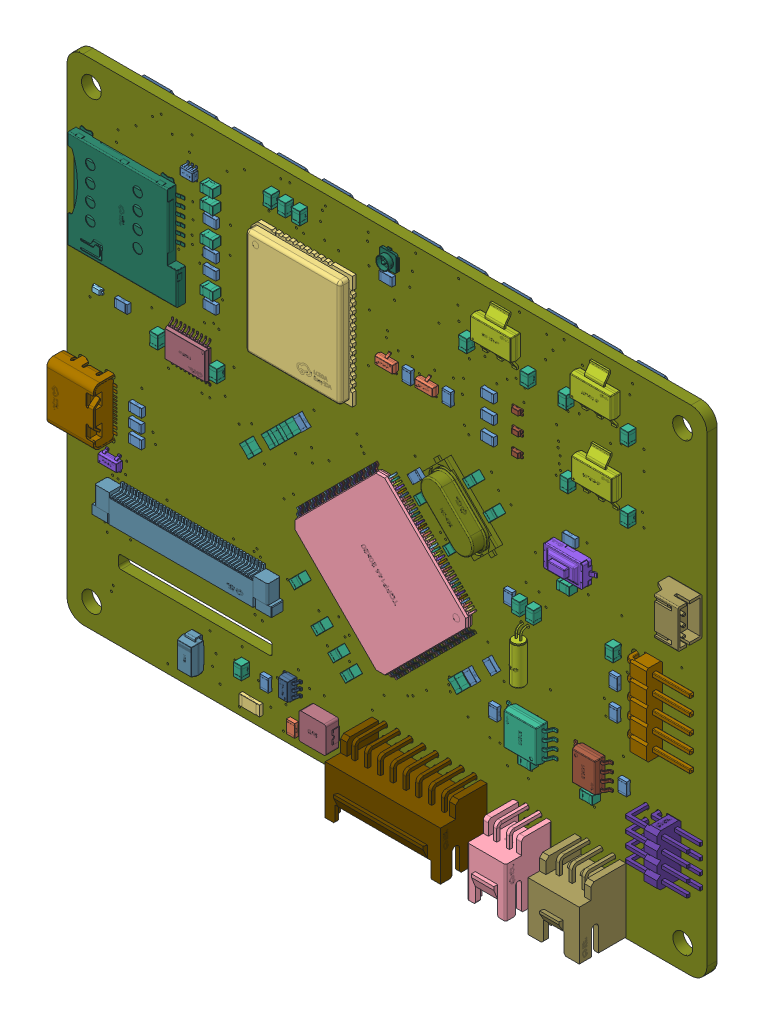
SolidWorks assembly steeringWheel_PCBA_v2.4, configuration 默认. Lengths in mm.
Overall size (100.05 77.22 11.5).
501 component instances, 178 part files, 0 mates.
Components (placement in the parent):
- steeringWheel_PCBA_v2.4.step-1: steeringWheel_PCBA_v2.4.step [默认] at origin size (100.05 77.22 11.5)
  - R5.step-1: R5.step [默认] at (22.8608 -12.1785 1.6001) size (2 1.3 0.61)
    - R0805.step-1: R0805.step [默认] at origin size (2 1.3 0.61)
      - COMPOUND.step-1: COMPOUND.step [默认] at origin size (2 1.3 0.61)
  - R17.step-1: R17.step [默认] at (22.8608 -19.1262 1.6001) size (2 1.3 0.61)
    - R0805.step-1: R0805.step [默认] at origin size (2 1.3 0.61)
      - COMPOUND.step-1: COMPOUND.step [默认] at origin size (2 1.3 0.61)
  - R16.step-1: R16.step [默认] at (22.8608 -16.8013 1.6001) size (2 1.3 0.61)
    - R0805.step-1: R0805.step [默认] at origin size (2 1.3 0.61)
      - COMPOUND.step-1: COMPOUND.step [默认] at origin size (2 1.3 0.61)
  - R12.step-1: R12.step [默认] at (11.1969 -45.6947 1.6001) x (-1 0 0) z (0 0 1) size (2 1.3 0.61)
    - R0805.step-1: R0805.step [默认] at origin size (2 1.3 0.61)
      - COMPOUND.step-1: COMPOUND.step [默认] at origin size (2 1.3 0.61)
  - R13.step-1: R13.step [默认] at (11.2213 -47.7775 1.6001) x (-1 0 0) z (0 0 1) size (2 1.3 0.61)
    - R0805.step-1: R0805.step [默认] at origin size (2 1.3 0.61)
      - COMPOUND.step-1: COMPOUND.step [默认] at origin size (2 1.3 0.61)
  - R19.step-1: R19.step [默认] at (67.1323 -56.4887 1.6001) x (0 -1 0) z (0 0 1) size (2 1.3 0.61)
    - R0805.step-1: R0805.step [默认] at origin size (2 1.3 0.61)
      - COMPOUND.step-1: COMPOUND.step [默认] at origin size (2 1.3 0.61)
  - R39.step-1: R39.step [默认] at (54.8869 -30.762 1.6001) x (-0.707107 -0.707107 0) z (0 0 1) size (2 1.3 0.61)
    - R0805.step-1: R0805.step [默认] at origin size (2 1.3 0.61)
      - COMPOUND.step-1: COMPOUND.step [默认] at origin size (2 1.3 0.61)
  - R40.step-1: R40.step [默认] at (63.5255 -53.4925 1.6001) x (0.707107 -0.707107 0) z (0 0 1) size (2 1.3 0.61)
    - R0805.step-1: R0805.step [默认] at origin size (2 1.3 0.61)
      - COMPOUND.step-1: COMPOUND.step [默认] at origin size (2 1.3 0.61)
  - R1.step-1: R1.step [默认] at (78.9688 -27.3051 1.6001) size (2 1.3 0.61)
    - R0805.step-1: R0805.step [默认] at origin size (2 1.3 0.61)
      - COMPOUND.step-1: COMPOUND.step [默认] at origin size (2 1.3 0.61)
  - R8.step-1: R8.step [默认] at (31.3945 -70.4343 1.6001) x (0 1 0) z (0 0 1) size (2 1.3 0.61)
    - R0805.step-1: R0805.step [默认] at origin size (2 1.3 0.61)
      - COMPOUND.step-1: COMPOUND.step [默认] at origin size (2 1.3 0.61)
  - R9.step-1: R9.step [默认] at (22.8608 -23.749 1.6001) size (2 1.3 0.61)
    - R0805.step-1: R0805.step [默认] at origin size (2 1.3 0.61)
      - COMPOUND.step-1: COMPOUND.step [默认] at origin size (2 1.3 0.61)
  - R41.step-1: R41.step [默认] at (66.2475 -19.8882 1.6001) x (-1 0 0) z (0 0 1) size (2 1.3 0.61)
    - R0805.step-1: R0805.step [默认] at origin size (2 1.3 0.61)
      - COMPOUND.step-1: COMPOUND.step [默认] at origin size (2 1.3 0.61)
  - R10.step-1: R10.step [默认] at (66.2475 -16.9841 1.6001) x (-1 0 0) z (0 0 1) size (2 1.3 0.61)
    - R0805.step-1: R0805.step [默认] at origin size (2 1.3 0.61)
      - COMPOUND.step-1: COMPOUND.step [默认] at origin size (2 1.3 0.61)
  - R11.step-1: R11.step [默认] at (66.2475 -14.0716 1.6001) x (-1 0 0) z (0 0 1) size (2 1.3 0.61)
    - R0805.step-1: R0805.step [默认] at origin size (2 1.3 0.61)
      - COMPOUND.step-1: COMPOUND.step [默认] at origin size (2 1.3 0.61)
  - R14.step-1: R14.step [默认] at (50.3553 -6.1852 1.6001) x (-1 0 0) z (0 0 1) size (2 1.3 0.61)
    - R0805.step-1: R0805.step [默认] at origin size (2 1.3 0.61)
      - COMPOUND.step-1: COMPOUND.step [默认] at origin size (2 1.3 0.61)
  - R15.step-1: R15.step [默认] at (66.6497 -50.5207 1.6001) x (-0.707107 0.707107 0) z (0 0 1) size (2 1.3 0.61)
    - R0805.step-1: R0805.step [默认] at origin size (2 1.3 0.61)
      - COMPOUND.step-1: COMPOUND.step [默认] at origin size (2 1.3 0.61)
  - R18.step-1: R18.step [默认] at (37.0079 -32.3597 1.6001) x (0.707107 -0.707107 0) z (0 0 1) size (2 1.3 0.61)
    - R0805.step-1: R0805.step [默认] at origin size (2 1.3 0.61)
      - COMPOUND.step-1: COMPOUND.step [默认] at origin size (2 1.3 0.61)
  - R42.step-1: R42.step [默认] at (9.017 -30.5563 1.6001) size (2 1.3 0.61)
    - R0805.step-1: R0805.step [默认] at origin size (2 1.3 0.61)
      - COMPOUND.step-1: COMPOUND.step [默认] at origin size (2 1.3 0.61)
  - R20.step-1: R20.step [默认] at (69.4772 -39.7965 1.6001) x (0 1 0) z (0 0 1) size (2 1.3 0.61)
    - R0805.step-1: R0805.step [默认] at origin size (2 1.3 0.61)
      - COMPOUND.step-1: COMPOUND.step [默认] at origin size (2 1.3 0.61)
  - R43.step-1: R43.step [默认] at (11.2477 -43.4849 1.6001) size (2 1.3 0.61)
    - R0805.step-1: R0805.step [默认] at origin size (2 1.3 0.61)
      - COMPOUND.step-1: COMPOUND.step [默认] at origin size (2 1.3 0.61)
  - R44.step-1: R44.step [默认] at (53.6195 -17.7546 1.6001) x (0 1 0) z (0 0 1) size (2 1.3 0.61)
    - R0805.step-1: R0805.step [默认] at origin size (2 1.3 0.61)
      - COMPOUND.step-1: COMPOUND.step [默认] at origin size (2 1.3 0.61)
  - R21.step-1: R21.step [默认] at (59.8679 -17.526 1.6001) x (0 1 0) z (0 0 1) size (2 1.3 0.61)
    - R0805.step-1: R0805.step [默认] at origin size (2 1.3 0.61)
      - COMPOUND.step-1: COMPOUND.step [默认] at origin size (2 1.3 0.61)
  - L3.step-1: L3.step [默认] at (35.5347 -74.4729 1.6001) x (0 -1 0) z (0 0 1) size (2 1.3 0.61)
    - L0805.step-1: L0805.step [默认] at origin size (2 1.3 0.61)
      - COMPOUND-0.step-1: COMPOUND-0.step [默认] at origin size (2 1.3 0.61)
  - R22.step-1: R22.step [默认] at (85.9289 -42.9825 1.6001) x (0 -1 0) z (0 0 1) size (2 1.3 0.61)
    - R0805.step-1: R0805.step [默认] at origin size (2 1.3 0.61)
      - COMPOUND.step-1: COMPOUND.step [默认] at origin size (2 1.3 0.61)
  - R23.step-1: R23.step [默认] at (85.9035 -47.2497 1.6001) x (0 1 0) z (0 0 1) size (2 1.3 0.61)
    - R0805.step-1: R0805.step [默认] at origin size (2 1.3 0.61)
      - COMPOUND.step-1: COMPOUND.step [默认] at origin size (2 1.3 0.61)
  - R45.step-1: R45.step [默认] at (87.3762 -56.4643 1.6001) x (0 1 0) z (0 0 1) size (2 1.3 0.61)
    - R0805.step-1: R0805.step [默认] at origin size (2 1.3 0.61)
      - COMPOUND.step-1: COMPOUND.step [默认] at origin size (2 1.3 0.61)
  - R29.step-1: R29.step [默认] at (29.0323 -74.5745 1.6001) size (3.2 1.6 0.56)
    - R1206.step-1: R1206.step [默认] at origin size (3.2 1.6 0.56)
      - COMPOUND-1.step-1: COMPOUND-1.step [默认] at origin size (3.2 1.6 0.56)
  - BTN_INPUT.step-1: BTN_INPUT.step [默认] at (72.7457 -68.1991 1.6001) size (6 10.25 11)
    - CONN-TH_HX20028-4WAD.step-1: CONN-TH_HX20028-4WAD.step [默认] at origin size (6 10.25 11)
      - COMPOUND-2.step-1: COMPOUND-2.step [默认] at origin size (6 10.25 11)
  - LED.step-1: LED.step [默认] at (5.0419 -30.5283 1.6001) size (1.49 0.75 0.56)
    - LED0603-RD_BLUE.step-1: LED0603-RD_BLUE.step [默认] at origin size (1.49 0.75 0.56)
      - COMPOUND-3.step-1: COMPOUND-3.step [默认] at origin size (1.49 0.75 0.56)
  - C49.step-1: C49.step [默认] at (46.5187 -8.2909 0) x (-1 0 0) z (0 0 -1) size (2 1.3 1.3)
    - C0805.step-1: C0805.step [默认] at origin size (2 1.3 1.3)
      - SOLID.step-1: SOLID.step [默认] at origin size (2 1.3 1.3)
  - C48.step-1: C48.step [默认] at (39.4983 -8.2909 0) x (-1 0 0) z (0 0 -1) size (2 1.3 1.3)
    - C0805.step-1: C0805.step [默认] at origin size (2 1.3 1.3)
      - SOLID.step-1: SOLID.step [默认] at origin size (2 1.3 1.3)
  - C47.step-1: C47.step [默认] at (32.4778 -8.2909 0) x (-1 0 0) z (0 0 -1) size (2 1.3 1.3)
    - C0805.step-1: C0805.step [默认] at origin size (2 1.3 1.3)
      - SOLID.step-1: SOLID.step [默认] at origin size (2 1.3 1.3)
  - C46.step-1: C46.step [默认] at (25.4573 -8.2909 0) x (-1 0 0) z (0 0 -1) size (2 1.3 1.3)
    - C0805.step-1: C0805.step [默认] at origin size (2 1.3 1.3)
      - SOLID.step-1: SOLID.step [默认] at origin size (2 1.3 1.3)
  - C45.step-1: C45.step [默认] at (18.4368 -8.2909 0) x (-1 0 0) z (0 0 -1) size (2 1.3 1.3)
    - C0805.step-1: C0805.step [默认] at origin size (2 1.3 1.3)
      - SOLID.step-1: SOLID.step [默认] at origin size (2 1.3 1.3)
  - C44.step-1: C44.step [默认] at (11.4163 -8.2909 0) x (-1 0 0) z (0 0 -1) size (2 1.3 1.3)
    - C0805.step-1: C0805.step [默认] at origin size (2 1.3 1.3)
      - SOLID.step-1: SOLID.step [默认] at origin size (2 1.3 1.3)
  - C39.step-1: C39.step [默认] at (53.5392 -8.2909 0) x (1 0 0) z (0 0 -1) size (2 1.3 1.3)
    - C0805.step-1: C0805.step [默认] at origin size (2 1.3 1.3)
      - SOLID.step-1: SOLID.step [默认] at origin size (2 1.3 1.3)
  - C36.step-1: C36.step [默认] at (60.5597 -8.2909 0) x (1 0 0) z (0 0 -1) size (2 1.3 1.3)
    - C0805.step-1: C0805.step [默认] at origin size (2 1.3 1.3)
      - SOLID.step-1: SOLID.step [默认] at origin size (2 1.3 1.3)
  - C35.step-1: C35.step [默认] at (67.5802 -8.2909 0) x (1 0 0) z (0 0 -1) size (2 1.3 1.3)
    - C0805.step-1: C0805.step [默认] at origin size (2 1.3 1.3)
      - SOLID.step-1: SOLID.step [默认] at origin size (2 1.3 1.3)
  - C34.step-1: C34.step [默认] at (74.6007 -8.2909 0) x (1 0 0) z (0 0 -1) size (2 1.3 1.3)
    - C0805.step-1: C0805.step [默认] at origin size (2 1.3 1.3)
      - SOLID.step-1: SOLID.step [默认] at origin size (2 1.3 1.3)
  - C33.step-1: C33.step [默认] at (81.6212 -8.2909 0) x (1 0 0) z (0 0 -1) size (2 1.3 1.3)
    - C0805.step-1: C0805.step [默认] at origin size (2 1.3 1.3)
      - SOLID.step-1: SOLID.step [默认] at origin size (2 1.3 1.3)
  - C32.step-1: C32.step [默认] at (88.6417 -8.2909 0) x (1 0 0) z (0 0 -1) size (2 1.3 1.3)
    - C0805.step-1: C0805.step [默认] at origin size (2 1.3 1.3)
      - SOLID.step-1: SOLID.step [默认] at origin size (2 1.3 1.3)
  - C63.step-1: C63.step [默认] at (43.1547 -60.4013 1.6001) x (-0.707107 -0.707107 0) z (0 0 1) size (2 1.3 1.3)
    - C0805.step-1: C0805.step [默认] at origin size (2 1.3 1.3)
      - SOLID.step-1: SOLID.step [默认] at origin size (2 1.3 1.3)
  - C19.step-1: C19.step [默认] at (29.3879 -39.4971 1.6001) x (-0.707107 0.707107 0) z (0 0 1) size (2 1.3 1.3)
    - C0805.step-1: C0805.step [默认] at origin size (2 1.3 1.3)
      - SOLID.step-1: SOLID.step [默认] at origin size (2 1.3 1.3)
  - C67.step-1: C67.step [默认] at (78.6353 -8.2209 1.6001) x (0 1 0) z (0 0 1) size (2 1.3 1.3)
    - C0805.step-1: C0805.step [默认] at origin size (2 1.3 1.3)
      - SOLID.step-1: SOLID.step [默认] at origin size (2 1.3 1.3)
  - C4.step-1: C4.step [默认] at (45.0597 -62.2047 1.6001) x (0.707107 0.707107 0) z (0 0 1) size (2 1.3 1.3)
    - C0805.step-1: C0805.step [默认] at origin size (2 1.3 1.3)
      - SOLID.step-1: SOLID.step [默认] at origin size (2 1.3 1.3)
  - C5.step-1: C5.step [默认] at (40.5131 -58.0899 1.6001) x (0.707107 0.707107 0) z (0 0 1) size (2 1.3 1.3)
    - C0805.step-1: C0805.step [默认] at origin size (2 1.3 1.3)
      - SOLID.step-1: SOLID.step [默认] at origin size (2 1.3 1.3)
  - C6.step-1: C6.step [默认] at (37.0587 -53.5687 1.6001) x (0.707107 0.707107 0) z (0 0 1) size (2 1.3 1.3)
    - C0805.step-1: C0805.step [默认] at origin size (2 1.3 1.3)
      - SOLID.step-1: SOLID.step [默认] at origin size (2 1.3 1.3)
  - C7.step-1: C7.step [默认] at (61.0871 -37.0333 1.6001) x (-0.707107 -0.707107 0) z (0 0 1) size (2 1.3 1.3)
    - C0805.step-1: C0805.step [默认] at origin size (2 1.3 1.3)
      - SOLID.step-1: SOLID.step [默认] at origin size (2 1.3 1.3)
  - C8.step-1: C8.step [默认] at (56.5534 -32.5087 1.6001) x (-0.707107 -0.707107 0) z (0 0 1) size (2 1.3 1.3)
    - C0805.step-1: C0805.step [默认] at origin size (2 1.3 1.3)
      - SOLID.step-1: SOLID.step [默认] at origin size (2 1.3 1.3)
  - C9.step-1: C9.step [默认] at (32.768 -36.5382 1.6001) x (-0.707107 0.707107 0) z (0 0 1) size (2 1.3 1.3)
    - C0805.step-1: C0805.step [默认] at origin size (2 1.3 1.3)
      - SOLID.step-1: SOLID.step [默认] at origin size (2 1.3 1.3)
  - C10.step-1: C10.step [默认] at (34.1741 -35.1322 1.6001) x (-0.707107 0.707107 0) z (0 0 1) size (2 1.3 1.3)
    - C0805.step-1: C0805.step [默认] at origin size (2 1.3 1.3)
      - SOLID.step-1: SOLID.step [默认] at origin size (2 1.3 1.3)
  - C11.step-1: C11.step [默认] at (35.5802 -33.7261 1.6001) x (-0.707107 0.707107 0) z (0 0 1) size (2 1.3 1.3)
    - C0805.step-1: C0805.step [默认] at origin size (2 1.3 1.3)
      - SOLID.step-1: SOLID.step [默认] at origin size (2 1.3 1.3)
  - C2.step-1: C2.step [默认] at (88.3127 -8.3479 1.6001) x (0 1 0) z (0 0 1) size (2 1.3 1.3)
    - C0805.step-1: C0805.step [默认] at origin size (2 1.3 1.3)
      - SOLID.step-1: SOLID.step [默认] at origin size (2 1.3 1.3)
  - C13.step-1: C13.step [默认] at (61.9253 -55.0419 1.6001) x (-0.707107 0.707107 0) z (0 0 1) size (2 1.3 1.3)
    - C0805.step-1: C0805.step [默认] at origin size (2 1.3 1.3)
      - SOLID.step-1: SOLID.step [默认] at origin size (2 1.3 1.3)
  - C15.step-1: C15.step [默认] at (78.7656 -33.5027 1.6001) x (-1 0 0) z (0 0 1) size (2 1.3 1.3)
    - C0805.step-1: C0805.step [默认] at origin size (2 1.3 1.3)
      - SOLID.step-1: SOLID.step [默认] at origin size (2 1.3 1.3)
  - C18.step-1: C18.step [默认] at (78.9147 -19.3801 1.6001) x (0 1 0) z (0 0 1) size (2 1.3 1.3)
    - C0805.step-1: C0805.step [默认] at origin size (2 1.3 1.3)
      - SOLID.step-1: SOLID.step [默认] at origin size (2 1.3 1.3)
  - C25.step-1: C25.step [默认] at (88.2873 -19.3801 1.6001) x (0 -1 0) z (0 0 1) size (2 1.3 1.3)
    - C0805.step-1: C0805.step [默认] at origin size (2 1.3 1.3)
      - SOLID.step-1: SOLID.step [默认] at origin size (2 1.3 1.3)
  - C38.step-1: C38.step [默认] at (14.8336 -31.9672 1.6001) x (0 1 0) z (0 0 1) size (2 1.3 1.3)
    - C0805.step-1: C0805.step [默认] at origin size (2 1.3 1.3)
      - SOLID.step-1: SOLID.step [默认] at origin size (2 1.3 1.3)
  - C37.step-1: C37.step [默认] at (24.0792 -31.9164 1.6001) x (0 -1 0) z (0 0 1) size (2 1.3 1.3)
    - C0805.step-1: C0805.step [默认] at origin size (2 1.3 1.3)
      - SOLID.step-1: SOLID.step [默认] at origin size (2 1.3 1.3)
  - C31.step-1: C31.step [默认] at (63.1064 -8.3311 1.6001) x (0 -1 0) z (0 0 1) size (2 1.3 1.3)
    - C0805.step-1: C0805.step [默认] at origin size (2 1.3 1.3)
      - SOLID.step-1: SOLID.step [默认] at origin size (2 1.3 1.3)
  - C29.step-1: C29.step [默认] at (72.6822 -8.3311 1.6001) x (0 -1 0) z (0 0 1) size (2 1.3 1.3)
    - C0805.step-1: C0805.step [默认] at origin size (2 1.3 1.3)
      - SOLID.step-1: SOLID.step [默认] at origin size (2 1.3 1.3)
  - C41.step-1: C41.step [默认] at (32.5754 -4.1184 1.6001) x (0 -1 0) z (0 0 1) size (2 1.3 1.3)
    - C0805.step-1: C0805.step [默认] at origin size (2 1.3 1.3)
      - SOLID.step-1: SOLID.step [默认] at origin size (2 1.3 1.3)
  - C40.step-1: C40.step [默认] at (34.7859 -4.1184 1.6001) x (0 -1 0) z (0 0 1) size (2 1.3 1.3)
    - C0805.step-1: C0805.step [默认] at origin size (2 1.3 1.3)
      - SOLID.step-1: SOLID.step [默认] at origin size (2 1.3 1.3)
  - C50.step-1: C50.step [默认] at (23.0632 -7.5692 1.6001) size (2 1.3 1.3)
    - C0805.step-1: C0805.step [默认] at origin size (2 1.3 1.3)
      - SOLID.step-1: SOLID.step [默认] at origin size (2 1.3 1.3)
  - C43.step-1: C43.step [默认] at (72.6949 -60.1473 1.6001) x (-1 0 0) z (0 0 1) size (2 1.3 1.3)
    - C0805.step-1: C0805.step [默认] at origin size (2 1.3 1.3)
      - SOLID.step-1: SOLID.step [默认] at origin size (2 1.3 1.3)
  - C17.step-1: C17.step [默认] at (36.9963 -4.1184 1.6001) x (0 -1 0) z (0 0 1) size (2 1.3 1.3)
    - C0805.step-1: C0805.step [默认] at origin size (2 1.3 1.3)
      - SOLID.step-1: SOLID.step [默认] at origin size (2 1.3 1.3)
  - C69.step-1: C69.step [默认] at (23.0632 -14.4899 1.6001) x (-1 0 0) z (0 0 1) size (2 1.3 1.3)
    - C0805.step-1: C0805.step [默认] at origin size (2 1.3 1.3)
      - SOLID.step-1: SOLID.step [默认] at origin size (2 1.3 1.3)
  - C21.step-1: C21.step [默认] at (23.0632 -21.4376 1.6001) x (-1 0 0) z (0 0 1) size (2 1.3 1.3)
    - C0805.step-1: C0805.step [默认] at origin size (2 1.3 1.3)
      - SOLID.step-1: SOLID.step [默认] at origin size (2 1.3 1.3)
  - C22.step-1: C22.step [默认] at (23.0632 -9.8671 1.6001) x (-1 0 0) z (0 0 1) size (2 1.3 1.3)
    - C0805.step-1: C0805.step [默认] at origin size (2 1.3 1.3)
      - SOLID.step-1: SOLID.step [默认] at origin size (2 1.3 1.3)
  - C70.step-1: C70.step [默认] at (73.5412 -39.8473 1.6001) x (0 1 0) z (0 0 1) size (2 1.3 1.3)
    - C0805.step-1: C0805.step [默认] at origin size (2 1.3 1.3)
      - SOLID.step-1: SOLID.step [默认] at origin size (2 1.3 1.3)
  - C71.step-1: C71.step [默认] at (71.3568 -39.8219 1.6001) x (0 1 0) z (0 0 1) size (2 1.3 1.3)
    - C0805.step-1: C0805.step [默认] at origin size (2 1.3 1.3)
      - SOLID.step-1: SOLID.step [默认] at origin size (2 1.3 1.3)
  - C72.step-1: C72.step [默认] at (27.9147 -70.1803 1.6001) x (0 -1 0) z (0 0 1) size (2 1.3 1.3)
    - C0805.step-1: C0805.step [默认] at origin size (2 1.3 1.3)
      - SOLID.step-1: SOLID.step [默认] at origin size (2 1.3 1.3)
  - C20.step-1: C20.step [默认] at (85.9792 -38.7211 1.6001) x (0 -1 0) z (0 0 1) size (2 1.3 1.3)
    - C0805.step-1: C0805.step [默认] at origin size (2 1.3 1.3)
      - SOLID.step-1: SOLID.step [默认] at origin size (2 1.3 1.3)
  - C73.step-1: C73.step [默认] at (67.4371 -29.3117 1.6001) x (0.707107 0.707107 0) z (0 0 1) size (2 1.3 1.3)
    - C0805.step-1: C0805.step [默认] at origin size (2 1.3 1.3)
      - SOLID.step-1: SOLID.step [默认] at origin size (2 1.3 1.3)
  - C16.step-1: C16.step [默认] at (64.2072 -26.3439 1.6001) x (0.707107 0.707107 0) z (0 0 1) size (2 1.3 1.3)
    - C0805.step-1: C0805.step [默认] at origin size (2 1.3 1.3)
      - SOLID.step-1: SOLID.step [默认] at origin size (2 1.3 1.3)
  - C51.step-1: C51.step [默认] at (82.3724 -59.9949 1.6001) size (2 1.3 1.3)
    - C0805.step-1: C0805.step [默认] at origin size (2 1.3 1.3)
      - SOLID.step-1: SOLID.step [默认] at origin size (2 1.3 1.3)
  - 32.768K.step-1: 32.768K.step [默认] at (71.5346 -42.6667 1.6001) x (0 1 0) z (0 0 1) size (7.62 2 5.52)
    - OSC-TH_BD2.0-P0.70-D0.3.step-1: OSC-TH_BD2.0-P0.70-D0.3.step [默认] at origin size (7.62 2 5.52)
      - SOLID-4.step-1: SOLID-4.step [默认] at origin size (7.62 2 5.52)
  - K2.step-1: K2.step [默认] at (78.9716 -30.3247 1.6001) size (7.9 3.6 2.6)
    - SW-SMD_L6.1-W3.6-LS8.0.step-1: SW-SMD_L6.1-W3.6-LS8.0.step [默认] at origin size (7.9 3.6 2.6)
      - COMPOUND-5.step-1: COMPOUND-5.step [默认] at origin size (7.9 3.6 2.6)
  - LINK.step-1: LINK.step [默认] at (88.7732 -43.0531 1.6001) x (0 -1 0) z (0 0 1) size (12.7 10.36 5.54)
    - HDR-TH_5P-P2.54-H-M-W10.0-N.step-1: HDR-TH_5P-P2.54-H-M-W10.0-N.step [默认] at origin size (12.7 10.36 5.54)
      - SOLID-6.step-1: SOLID-6.step [默认] at origin size (12.7 10.36 5.54)
  - LED1.step-1: LED1.step [默认] at (88.6423 -3.7019 0) x (1 0 0) z (0 0 -1) size (5.4 5.01 1.57)
    - LED-SMD_4P-L5.0-W5.0-TL_WS2812B-B.step-1: LED-SMD_4P-L5.0-W5.0-TL_WS2812B-B.step [默认] at origin size (5.4 5.01 1.57)
      - SOLID-7.step-1: SOLID-7.step [默认] at origin size (5.4 5.01 1.57)
  - LED4.step-1: LED4.step [默认] at (67.5807 -3.7019 0) x (1 0 0) z (0 0 -1) size (5.4 5.01 1.57)
    - LED-SMD_4P-L5.0-W5.0-TL_WS2812B-B.step-1: LED-SMD_4P-L5.0-W5.0-TL_WS2812B-B.step [默认] at origin size (5.4 5.01 1.57)
      - SOLID-7.step-1: SOLID-7.step [默认] at origin size (5.4 5.01 1.57)
  - LED5.step-1: LED5.step [默认] at (60.5601 -3.7019 0) x (1 0 0) z (0 0 -1) size (5.4 5.01 1.57)
    - LED-SMD_4P-L5.0-W5.0-TL_WS2812B-B.step-1: LED-SMD_4P-L5.0-W5.0-TL_WS2812B-B.step [默认] at origin size (5.4 5.01 1.57)
      - SOLID-7.step-1: SOLID-7.step [默认] at origin size (5.4 5.01 1.57)
  - LED7.step-1: LED7.step [默认] at (46.519 -3.7019 0) x (1 0 0) z (0 0 -1) size (5.4 5.01 1.57)
    - LED-SMD_4P-L5.0-W5.0-TL_WS2812B-B.step-1: LED-SMD_4P-L5.0-W5.0-TL_WS2812B-B.step [默认] at origin size (5.4 5.01 1.57)
      - SOLID-7.step-1: SOLID-7.step [默认] at origin size (5.4 5.01 1.57)
  - LED11.step-1: LED11.step [默认] at (18.4368 -3.7019 0) x (1 0 0) z (0 0 -1) size (5.4 5.01 1.57)
    - LED-SMD_4P-L5.0-W5.0-TL_WS2812B-B.step-1: LED-SMD_4P-L5.0-W5.0-TL_WS2812B-B.step [默认] at origin size (5.4 5.01 1.57)
      - SOLID-7.step-1: SOLID-7.step [默认] at origin size (5.4 5.01 1.57)
  - LED3.step-1: LED3.step [默认] at (74.6012 -3.7019 0) x (1 0 0) z (0 0 -1) size (5.4 5.01 1.57)
    - LED-SMD_4P-L5.0-W5.0-TL_WS2812B-B.step-1: LED-SMD_4P-L5.0-W5.0-TL_WS2812B-B.step [默认] at origin size (5.4 5.01 1.57)
      - SOLID-7.step-1: SOLID-7.step [默认] at origin size (5.4 5.01 1.57)
  - LED10.step-1: LED10.step [默认] at (25.4574 -3.7019 0) x (1 0 0) z (0 0 -1) size (5.4 5.01 1.57)
    - LED-SMD_4P-L5.0-W5.0-TL_WS2812B-B.step-1: LED-SMD_4P-L5.0-W5.0-TL_WS2812B-B.step [默认] at origin size (5.4 5.01 1.57)
      - SOLID-7.step-1: SOLID-7.step [默认] at origin size (5.4 5.01 1.57)
  - LED12.step-1: LED12.step [默认] at (11.4163 -3.7019 0) x (1 0 0) z (0 0 -1) size (5.4 5.01 1.57)
    - LED-SMD_4P-L5.0-W5.0-TL_WS2812B-B.step-1: LED-SMD_4P-L5.0-W5.0-TL_WS2812B-B.step [默认] at origin size (5.4 5.01 1.57)
      - SOLID-7.step-1: SOLID-7.step [默认] at origin size (5.4 5.01 1.57)
  - LED6.step-1: LED6.step [默认] at (53.5396 -3.7019 0) x (1 0 0) z (0 0 -1) size (5.4 5.01 1.57)
    - LED-SMD_4P-L5.0-W5.0-TL_WS2812B-B.step-1: LED-SMD_4P-L5.0-W5.0-TL_WS2812B-B.step [默认] at origin size (5.4 5.01 1.57)
      - SOLID-7.step-1: SOLID-7.step [默认] at origin size (5.4 5.01 1.57)
  - LED8.step-1: LED8.step [默认] at (39.4985 -3.7019 0) x (1 0 0) z (0 0 -1) size (5.4 5.01 1.57)
    - LED-SMD_4P-L5.0-W5.0-TL_WS2812B-B.step-1: LED-SMD_4P-L5.0-W5.0-TL_WS2812B-B.step [默认] at origin size (5.4 5.01 1.57)
      - SOLID-7.step-1: SOLID-7.step [默认] at origin size (5.4 5.01 1.57)
  - LED9.step-1: LED9.step [默认] at (32.4779 -3.7019 0) x (1 0 0) z (0 0 -1) size (5.4 5.01 1.57)
    - LED-SMD_4P-L5.0-W5.0-TL_WS2812B-B.step-1: LED-SMD_4P-L5.0-W5.0-TL_WS2812B-B.step [默认] at origin size (5.4 5.01 1.57)
      - SOLID-7.step-1: SOLID-7.step [默认] at origin size (5.4 5.01 1.57)
  - LED2.step-1: LED2.step [默认] at (81.6218 -3.7019 0) x (1 0 0) z (0 0 -1) size (5.4 5.01 1.57)
    - LED-SMD_4P-L5.0-W5.0-TL_WS2812B-B.step-1: LED-SMD_4P-L5.0-W5.0-TL_WS2812B-B.step [默认] at origin size (5.4 5.01 1.57)
      - SOLID-7.step-1: SOLID-7.step [默认] at origin size (5.4 5.01 1.57)
  - LED2-1.step-1: LED2-1.step [默认] at (70.4851 -19.9136 1.6001) size (1.62 0.82 0.56)
    - LED0603-RD.step-1: LED0603-RD.step [默认] at origin size (1.62 0.82 0.56)
      - COMPOUND-8.step-1: COMPOUND-8.step [默认] at origin size (1.62 0.82 0.56)
  - LED1-1.step-1: LED1-1.step [默认] at (70.5359 -16.9418 1.6001) size (1.62 0.82 0.56)
    - LED0603-RD.step-1: LED0603-RD.step [默认] at origin size (1.62 0.82 0.56)
      - COMPOUND-8.step-1: COMPOUND-8.step [默认] at origin size (1.62 0.82 0.56)
  - LED_P.step-1: LED_P.step [默认] at (70.5105 -14.1224 1.6001) size (1.62 0.82 0.56)
    - LED0603-RD.step-1: LED0603-RD.step [默认] at origin size (1.62 0.82 0.56)
      - COMPOUND-8.step-1: COMPOUND-8.step [默认] at origin size (1.62 0.82 0.56)
  - USB&CAN.step-1: USB&CAN.step [默认] at (83.3376 -68.0975 1.6001) size (8 10.25 11.2)
    - CONN-TH_M2026R-2X3P.step-1: CONN-TH_M2026R-2X3P.step [默认] at origin size (8 10.25 11.2)
      - COMPOUND-9.step-1: COMPOUND-9.step [默认] at origin size (8 10.25 11.2)
  - L5.step-1: L5.step [默认] at (40.4623 -71.8567 1.6001) x (-1 0 0) z (0 0 1) size (4.41 4.2 2.1)
    - IND-SMD_L4.4-W4.2.step-1: IND-SMD_L4.4-W4.2.step [默认] at origin size (4.41 4.2 2.1)
      - SOLID-10.step-1: SOLID-10.step [默认] at origin size (4.41 4.2 2.1)
  - D5.step-1: D5.step [默认] at (20.4216 -71.7805 1.6001) x (0 -1 0) z (0 0 1) size (5.2 2.5 2.1)
    - SMA_L4.4-W2.6-LS5.0-RD.step-1: SMA_L4.4-W2.6-LS5.0-RD.step [默认] at origin size (5.2 2.5 2.1)
      - COMPOUND-11.step-1: COMPOUND-11.step [默认] at origin size (5.2 2.5 2.1)
  - JP1.step-1: JP1.step [默认] at (50.4823 -3.0864 1.6001) x (0 -1 0) z (0 0 1) size (3.1 3 1.26)
    - ANT-SMD_UFL-R-SMT-1-10.step-1: ANT-SMD_UFL-R-SMT-1-10.step [默认] at origin size (3.1 3 1.26)
      - COMPOUND-12.step-1: COMPOUND-12.step [默认] at origin size (3.1 3 1.26)
  - X4.step-1: X4.step [默认] at (62.3825 -31.2167 1.6001) x (-0.707107 0.707107 0) z (0 0 1) size (12.7 4.8 3.11)
    - CRYSTAL-SMD_L11.5-W4.8-LS12.7.step-1: CRYSTAL-SMD_L11.5-W4.8-LS12.7.step [默认] at origin size (12.7 4.8 3.11)
      - COMPOUND-13.step-1: COMPOUND-13.step [默认] at origin size (12.7 4.8 3.11)
  - DEBUG.step-1: DEBUG.step [默认] at (91.491 -60.7569 1.6001) x (0 1 0) z (0 0 1) size (8.01 9.75 6.8)
    - HDR-TH_8P-P2.00-H-M-R2-C4-S2.00-W9.8.step-1: HDR-TH_8P-P2.00-H-M-R2-C4-S2.00-W9.8.step [默认] at origin size (8.01 9.75 6.8)
      - SOLID-14.step-1: SOLID-14.step [默认] at origin size (8.01 9.75 6.8)
  - KEY_INPUT.step-1: KEY_INPUT.step [默认] at (56.6421 -68.1483 1.6001) size (18 10.25 11.2)
    - CONN-TH_FWF20017-D16B22W5B.step-1: CONN-TH_FWF20017-D16B22W5B.step [默认] at origin size (18 10.25 11.2)
      - COMPOUND-15.step-1: COMPOUND-15.step [默认] at origin size (18 10.25 11.2)
  - D4.step-1: D4.step [默认] at (19.6342 -7.2644 1.6001) x (0 1 0) z (0 0 1) size (2.1 2 1)
    - SC-70-6_L2.2-W1.3-P0.65-LS2.1-BR.step-1: SC-70-6_L2.2-W1.3-P0.65-LS2.1-BR.step [默认] at origin size (2.1 2 1)
      - COMPOUND-16.step-1: COMPOUND-16.step [默认] at origin size (2.1 2 1)
  - Q4.step-1: Q4.step [默认] at (56.7437 -17.5514 1.6001) x (0 -1 0) z (0 0 1) size (2.5 2.89 1.05)
    - SOT-23-3_L2.9-W1.3-P1.90-LS2.4-BR.step-1: SOT-23-3_L2.9-W1.3-P1.90-LS2.4-BR.step [默认] at origin size (2.5 2.89 1.05)
      - COMPOUND-17.step-1: COMPOUND-17.step [默认] at origin size (2.5 2.89 1.05)
  - Q1.step-1: Q1.step [默认] at (50.4953 -17.5514 1.6001) x (0 -1 0) z (0 0 1) size (2.5 2.89 1.05)
    - SOT-23-3_L2.9-W1.3-P1.90-LS2.4-BR.step-1: SOT-23-3_L2.9-W1.3-P1.90-LS2.4-BR.step [默认] at origin size (2.5 2.89 1.05)
      - COMPOUND-17.step-1: COMPOUND-17.step [默认] at origin size (2.5 2.89 1.05)
  - BC260Y.step-1: BC260Y.step [默认] at (37.2873 -17.2974 1.6001) size (15.8 17.7 2.01)
    - LCC-LGA-58_L17.7-W15.8-P1.1-TL-BC260Y-CN.step-1: LCC-LGA-58_L17.7-W15.8-P1.1-TL-BC260Y-CN.step [默认] at origin size (15.8 17.7 2.01)
      - SOLID-18.step-1: SOLID-18.step [默认] at origin size (15.8 17.7 2.01)
  - STM32F407ZXT6.step-1: STM32F407ZXT6.step [默认] at (50.0293 -46.0772 1.6001) x (-0.707107 0.707107 0) z (0 0 1) size (22 22 1.06)
    - LQFP-144_L20.0-W20.0-P0.50-LS22.0-BL.step-1: LQFP-144_L20.0-W20.0-P0.50-LS22.0-BL.step [默认] at origin size (22 22 1.06)
      - SOLID-19.step-1: SOLID-19.step [默认] at origin size (20 20 1)
      - SOLID-20.step-1: SOLID-20.step [默认] at origin size (0.25 1 0.6)
      - SOLID-21.step-1: SOLID-21.step [默认] at origin size (0.25 1 0.6)
      - SOLID-22.step-1: SOLID-22.step [默认] at origin size (0.25 1 0.6)
      - SOLID-23.step-1: SOLID-23.step [默认] at origin size (0.25 1 0.6)
      - SOLID-24.step-1: SOLID-24.step [默认] at origin size (0.25 1 0.6)
      - SOLID-25.step-1: SOLID-25.step [默认] at origin size (0.25 1 0.6)
      - SOLID-26.step-1: SOLID-26.step [默认] at origin size (0.25 1 0.6)
      - SOLID-27.step-1: SOLID-27.step [默认] at origin size (0.25 1 0.6)
      - SOLID-28.step-1: SOLID-28.step [默认] at origin size (0.25 1 0.6)
      - SOLID-29.step-1: SOLID-29.step [默认] at origin size (0.25 1 0.6)
      - SOLID-30.step-1: SOLID-30.step [默认] at origin size (0.25 1 0.6)
      - SOLID-31.step-1: SOLID-31.step [默认] at origin size (0.25 1 0.6)
      - SOLID-32.step-1: SOLID-32.step [默认] at origin size (0.25 1 0.6)
      - SOLID-33.step-1: SOLID-33.step [默认] at origin size (0.25 1 0.6)
      - SOLID-34.step-1: SOLID-34.step [默认] at origin size (0.25 1 0.6)
      - SOLID-35.step-1: SOLID-35.step [默认] at origin size (0.25 1 0.6)
      - SOLID-36.step-1: SOLID-36.step [默认] at origin size (0.25 1 0.6)
      - SOLID-37.step-1: SOLID-37.step [默认] at origin size (0.25 1 0.6)
      - SOLID-38.step-1: SOLID-38.step [默认] at origin size (0.25 1 0.6)
      - SOLID-39.step-1: SOLID-39.step [默认] at origin size (0.25 1 0.6)
      - SOLID-40.step-1: SOLID-40.step [默认] at origin size (0.25 1 0.6)
      - SOLID-41.step-1: SOLID-41.step [默认] at origin size (0.25 1 0.6)
      - SOLID-42.step-1: SOLID-42.step [默认] at origin size (0.25 1 0.6)
      - SOLID-43.step-1: SOLID-43.step [默认] at origin size (0.25 1 0.6)
      - SOLID-44.step-1: SOLID-44.step [默认] at origin size (0.25 1 0.6)
      - SOLID-45.step-1: SOLID-45.step [默认] at origin size (0.25 1 0.6)
      - SOLID-46.step-1: SOLID-46.step [默认] at origin size (0.25 1 0.6)
      - SOLID-47.step-1: SOLID-47.step [默认] at origin size (0.25 1 0.6)
      - SOLID-48.step-1: SOLID-48.step [默认] at origin size (0.25 1 0.6)
      - SOLID-49.step-1: SOLID-49.step [默认] at origin size (0.25 1 0.6)
      - SOLID-50.step-1: SOLID-50.step [默认] at origin size (0.25 1 0.6)
      - SOLID-51.step-1: SOLID-51.step [默认] at origin size (0.25 1 0.6)
      - SOLID-52.step-1: SOLID-52.step [默认] at origin size (0.25 1 0.6)
      - SOLID-53.step-1: SOLID-53.step [默认] at origin size (0.25 1 0.6)
      - SOLID-54.step-1: SOLID-54.step [默认] at origin size (0.25 1 0.6)
      - SOLID-55.step-1: SOLID-55.step [默认] at origin size (0.25 1 0.6)
      - SOLID-56.step-1: SOLID-56.step [默认] at origin size (1 0.25 0.6)
      - SOLID-57.step-1: SOLID-57.step [默认] at origin size (0.25 1 0.6)
      - SOLID-58.step-1: SOLID-58.step [默认] at origin size (1 0.25 0.6)
      - SOLID-59.step-1: SOLID-59.step [默认] at origin size (1 0.25 0.6)
      - SOLID-60.step-1: SOLID-60.step [默认] at origin size (0.25 1 0.6)
      - SOLID-61.step-1: SOLID-61.step [默认] at origin size (1 0.25 0.6)
      - SOLID-62.step-1: SOLID-62.step [默认] at origin size (1 0.25 0.6)
      - SOLID-63.step-1: SOLID-63.step [默认] at origin size (0.25 1 0.6)
      - SOLID-64.step-1: SOLID-64.step [默认] at origin size (1 0.25 0.6)
      - SOLID-65.step-1: SOLID-65.step [默认] at origin size (1 0.25 0.6)
      - SOLID-66.step-1: SOLID-66.step [默认] at origin size (0.25 1 0.6)
      - SOLID-67.step-1: SOLID-67.step [默认] at origin size (1 0.25 0.6)
      - SOLID-68.step-1: SOLID-68.step [默认] at origin size (1 0.25 0.6)
      - SOLID-69.step-1: SOLID-69.step [默认] at origin size (0.25 1 0.6)
      - SOLID-70.step-1: SOLID-70.step [默认] at origin size (1 0.25 0.6)
      - SOLID-71.step-1: SOLID-71.step [默认] at origin size (1 0.25 0.6)
      - SOLID-72.step-1: SOLID-72.step [默认] at origin size (0.25 1 0.6)
      - SOLID-73.step-1: SOLID-73.step [默认] at origin size (1 0.25 0.6)
      - SOLID-74.step-1: SOLID-74.step [默认] at origin size (1 0.25 0.6)
      - SOLID-75.step-1: SOLID-75.step [默认] at origin size (0.25 1 0.6)
      - SOLID-76.step-1: SOLID-76.step [默认] at origin size (1 0.25 0.6)
      - SOLID-77.step-1: SOLID-77.step [默认] at origin size (1 0.25 0.6)
      - SOLID-78.step-1: SOLID-78.step [默认] at origin size (0.25 1 0.6)
      - SOLID-79.step-1: SOLID-79.step [默认] at origin size (1 0.25 0.6)
      - SOLID-80.step-1: SOLID-80.step [默认] at origin size (1 0.25 0.6)
      - SOLID-81.step-1: SOLID-81.step [默认] at origin size (0.25 1 0.6)
      - SOLID-82.step-1: SOLID-82.step [默认] at origin size (1 0.25 0.6)
      - SOLID-83.step-1: SOLID-83.step [默认] at origin size (1 0.25 0.6)
      - SOLID-84.step-1: SOLID-84.step [默认] at origin size (0.25 1 0.6)
      - SOLID-85.step-1: SOLID-85.step [默认] at origin size (1 0.25 0.6)
      - SOLID-86.step-1: SOLID-86.step [默认] at origin size (1 0.25 0.6)
      - SOLID-87.step-1: SOLID-87.step [默认] at origin size (0.25 1 0.6)
      - SOLID-88.step-1: SOLID-88.step [默认] at origin size (1 0.25 0.6)
      - SOLID-89.step-1: SOLID-89.step [默认] at origin size (1 0.25 0.6)
      - SOLID-90.step-1: SOLID-90.step [默认] at origin size (0.25 1 0.6)
      - SOLID-91.step-1: SOLID-91.step [默认] at origin size (1 0.25 0.6)
      - SOLID-92.step-1: SOLID-92.step [默认] at origin size (1 0.25 0.6)
      - SOLID-93.step-1: SOLID-93.step [默认] at origin size (0.25 1 0.6)
      - SOLID-94.step-1: SOLID-94.step [默认] at origin size (1 0.25 0.6)
      - SOLID-95.step-1: SOLID-95.step [默认] at origin size (1 0.25 0.6)
      - SOLID-96.step-1: SOLID-96.step [默认] at origin size (0.25 1 0.6)
      - SOLID-97.step-1: SOLID-97.step [默认] at origin size (1 0.25 0.6)
      - SOLID-98.step-1: SOLID-98.step [默认] at origin size (1 0.25 0.6)
      - SOLID-99.step-1: SOLID-99.step [默认] at origin size (0.25 1 0.6)
      - SOLID-100.step-1: SOLID-100.step [默认] at origin size (1 0.25 0.6)
      - SOLID-101.step-1: SOLID-101.step [默认] at origin size (1 0.25 0.6)
      - SOLID-102.step-1: SOLID-102.step [默认] at origin size (0.25 1 0.6)
      - SOLID-103.step-1: SOLID-103.step [默认] at origin size (1 0.25 0.6)
      - SOLID-104.step-1: SOLID-104.step [默认] at origin size (1 0.25 0.6)
      - SOLID-105.step-1: SOLID-105.step [默认] at origin size (0.25 1 0.6)
      - SOLID-106.step-1: SOLID-106.step [默认] at origin size (1 0.25 0.6)
      - SOLID-107.step-1: SOLID-107.step [默认] at origin size (1 0.25 0.6)
      - SOLID-108.step-1: SOLID-108.step [默认] at origin size (0.25 1 0.6)
      - SOLID-109.step-1: SOLID-109.step [默认] at origin size (1 0.25 0.6)
      - SOLID-110.step-1: SOLID-110.step [默认] at origin size (1 0.25 0.6)
      - SOLID-111.step-1: SOLID-111.step [默认] at origin size (0.25 1 0.6)
      - SOLID-112.step-1: SOLID-112.step [默认] at origin size (1 0.25 0.6)
      - SOLID-113.step-1: SOLID-113.step [默认] at origin size (1 0.25 0.6)
      - SOLID-114.step-1: SOLID-114.step [默认] at origin size (0.25 1 0.6)
      - SOLID-115.step-1: SOLID-115.step [默认] at origin size (1 0.25 0.6)
      - SOLID-116.step-1: SOLID-116.step [默认] at origin size (1 0.25 0.6)
      - SOLID-117.step-1: SOLID-117.step [默认] at origin size (0.25 1 0.6)
      - SOLID-118.step-1: SOLID-118.step [默认] at origin size (1 0.25 0.6)
      - SOLID-119.step-1: SOLID-119.step [默认] at origin size (1 0.25 0.6)
      - SOLID-120.step-1: SOLID-120.step [默认] at origin size (0.25 1 0.6)
      - SOLID-121.step-1: SOLID-121.step [默认] at origin size (1 0.25 0.6)
      - SOLID-122.step-1: SOLID-122.step [默认] at origin size (1 0.25 0.6)
      - SOLID-123.step-1: SOLID-123.step [默认] at origin size (0.25 1 0.6)
      - SOLID-124.step-1: SOLID-124.step [默认] at origin size (1 0.25 0.6)
      - SOLID-125.step-1: SOLID-125.step [默认] at origin size (1 0.25 0.6)
      - SOLID-126.step-1: SOLID-126.step [默认] at origin size (0.25 1 0.6)
      - SOLID-127.step-1: SOLID-127.step [默认] at origin size (1 0.25 0.6)
      - SOLID-128.step-1: SOLID-128.step [默认] at origin size (1 0.25 0.6)
      - SOLID-129.step-1: SOLID-129.step [默认] at origin size (0.25 1 0.6)
      - SOLID-130.step-1: SOLID-130.step [默认] at origin size (1 0.25 0.6)
      - SOLID-131.step-1: SOLID-131.step [默认] at origin size (1 0.25 0.6)
      - SOLID-132.step-1: SOLID-132.step [默认] at origin size (0.25 1 0.6)
      - SOLID-133.step-1: SOLID-133.step [默认] at origin size (1 0.25 0.6)
      - SOLID-134.step-1: SOLID-134.step [默认] at origin size (1 0.25 0.6)
      - SOLID-135.step-1: SOLID-135.step [默认] at origin size (0.25 1 0.6)
      - SOLID-136.step-1: SOLID-136.step [默认] at origin size (1 0.25 0.6)
      - SOLID-137.step-1: SOLID-137.step [默认] at origin size (1 0.25 0.6)
      - SOLID-138.step-1: SOLID-138.step [默认] at origin size (0.25 1 0.6)
      - SOLID-139.step-1: SOLID-139.step [默认] at origin size (1 0.25 0.6)
      - SOLID-140.step-1: SOLID-140.step [默认] at origin size (1 0.25 0.6)
      - SOLID-141.step-1: SOLID-141.step [默认] at origin size (0.25 1 0.6)
      - SOLID-142.step-1: SOLID-142.step [默认] at origin size (1 0.25 0.6)
      - SOLID-143.step-1: SOLID-143.step [默认] at origin size (1 0.25 0.6)
      - SOLID-144.step-1: SOLID-144.step [默认] at origin size (0.25 1 0.6)
      - SOLID-145.step-1: SOLID-145.step [默认] at origin size (1 0.25 0.6)
      - SOLID-146.step-1: SOLID-146.step [默认] at origin size (1 0.25 0.6)
      - SOLID-147.step-1: SOLID-147.step [默认] at origin size (0.25 1 0.6)
      - SOLID-148.step-1: SOLID-148.step [默认] at origin size (1 0.25 0.6)
      - SOLID-149.step-1: SOLID-149.step [默认] at origin size (1 0.25 0.6)
      - SOLID-150.step-1: SOLID-150.step [默认] at origin size (0.25 1 0.6)
      - SOLID-151.step-1: SOLID-151.step [默认] at origin size (1 0.25 0.6)
      - SOLID-152.step-1: SOLID-152.step [默认] at origin size (1 0.25 0.6)
      - SOLID-153.step-1: SOLID-153.step [默认] at origin size (0.25 1 0.6)
      - SOLID-154.step-1: SOLID-154.step [默认] at origin size (1 0.25 0.6)
      - SOLID-155.step-1: SOLID-155.step [默认] at origin size (1 0.25 0.6)
      - SOLID-156.step-1: SOLID-156.step [默认] at origin size (0.25 1 0.6)
      - SOLID-157.step-1: SOLID-157.step [默认] at origin size (1 0.25 0.6)
      - SOLID-158.step-1: SOLID-158.step [默认] at origin size (1 0.25 0.6)
      - SOLID-159.step-1: SOLID-159.step [默认] at origin size (0.25 1 0.6)
      - SOLID-160.step-1: SOLID-160.step [默认] at origin size (1 0.25 0.6)
      - SOLID-161.step-1: SOLID-161.step [默认] at origin size (1 0.25 0.6)
      - SOLID-162.step-1: SOLID-162.step [默认] at origin size (0.25 1 0.6)
      - SOLID-163.step-1: SOLID-163.step [默认] at origin size (1 0.25 0.6)
      - COMPOUND-164.step-1: COMPOUND-164.step [默认] at origin size (2.25 2.6 0.01)
  - FLASH.step-1: FLASH.step [默认] at (72.8142 -56.3571 1.6001) x (0 1 0) z (0 0 1) size (5.3 7.91 2.07)
    - SOIC-8_L5.3-W5.3-P1.27-LS8.0-BL.step-1: SOIC-8_L5.3-W5.3-P1.27-LS8.0-BL.step [默认] at origin size (5.3 7.91 2.07)
      - COMPOUND-165.step-1: COMPOUND-165.step [默认] at origin size (5.3 7.91 2.07)
  - U6.step-1: U6.step [默认] at (83.4646 -5.1816 1.6001) x (0 -1 0) z (0 0 1) size (7.11 6.5 1.75)
    - SOT-223-3_L6.5-W3.4-P2.30-LS7.0-BR.step-1: SOT-223-3_L6.5-W3.4-P2.30-LS7.0-BR.step [默认] at origin size (7.11 6.5 1.75)
      - COMPOUND-166.step-1: COMPOUND-166.step [默认] at origin size (7.11 6.5 1.75)
  - U3.step-1: U3.step [默认] at (67.8943 -5.1308 1.6001) x (0 -1 0) z (0 0 1) size (7.11 6.5 1.75)
    - SOT-223-3_L6.5-W3.4-P2.30-LS7.0-BR.step-1: SOT-223-3_L6.5-W3.4-P2.30-LS7.0-BR.step [默认] at origin size (7.11 6.5 1.75)
      - COMPOUND-166.step-1: COMPOUND-166.step [默认] at origin size (7.11 6.5 1.75)
  - U1.step-1: U1.step [默认] at (83.6932 -16.2306 1.6001) x (0 -1 0) z (0 0 1) size (7.11 6.5 1.75)
    - SOT-223-3_L6.5-W3.4-P2.30-LS7.0-BR.step-1: SOT-223-3_L6.5-W3.4-P2.30-LS7.0-BR.step [默认] at origin size (7.11 6.5 1.75)
      - COMPOUND-166.step-1: COMPOUND-166.step [默认] at origin size (7.11 6.5 1.75)
  - D7.step-1: D7.step [默认] at (7.366 -52.4003 1.6001) size (3 2.31 1.1)
    - SOT-143_L2.9-W1.3-P1.92-LS2.3-BL.step-1: SOT-143_L2.9-W1.3-P1.92-LS2.3-BL.step [默认] at origin size (3 2.31 1.1)
      - COMPOUND-167.step-1: COMPOUND-167.step [默认] at origin size (3 2.31 1.1)
  - USB.step-1: USB.step [默认] at (5.0237 -45.5423 1.6001) x (0 -1 0) z (0 0 1) size (8.94 7.9 4.1)
    - USB-C_SMD-TYPE-C-31-M-12.step-1: USB-C_SMD-TYPE-C-31-M-12.step [默认] at origin size (8.94 7.9 4.1)
      - COMPOUND-168.step-1: COMPOUND-168.step [默认] at origin size (8.94 7.9 4.1)
  - U10.step-1: U10.step [默认] at (35.3823 -68.7833 1.6001) size (2.81 2.9 1.65)
    - SOT-23-6_L2.9-W1.6-P0.95-LS2.8-BR.step-1: SOT-23-6_L2.9-W1.6-P0.95-LS2.8-BR.step [默认] at origin size (2.81 2.9 1.65)
      - COMPOUND-169.step-1: COMPOUND-169.step [默认] at origin size (2.81 2.9 1.65)
  - CAN.step-1: CAN.step [默认] at (82.3978 -56.3373 1.6001) x (0 -1 0) z (0 0 1) size (4.81 6 1.72)
    - SOIC-8_L5.0-W4.0-P1.27-LS6.0-BL.step-1: SOIC-8_L5.0-W4.0-P1.27-LS6.0-BL.step [默认] at origin size (4.81 6 1.72)
      - COMPOUND-170.step-1: COMPOUND-170.step [默认] at origin size (4.81 6 1.72)
  - ADJ.step-1: ADJ.step [默认] at (95.0724 -27.7115 1.6001) x (0 -1 0) z (0 0 1) size (6 5 6.4)
    - CONN-TH_S3B-ZR-LF-SN.step-1: CONN-TH_S3B-ZR-LF-SN.step [默认] at origin size (6 5 6.4)
      - COMPOUND-171.step-1: COMPOUND-171.step [默认] at origin size (6 5 6.4)
  - U13.step-1: U13.step [默认] at (19.4819 -31.7381 1.6001) x (-1 0 0) z (0 0 1) size (6.49 6.4 1.05)
    - TSSOP-20_L6.5-W4.4-P0.65-LS6.4-BL.step-1: TSSOP-20_L6.5-W4.4-P0.65-LS6.4-BL.step [默认] at origin size (6.49 6.4 1.05)
      - COMPOUND-172.step-1: COMPOUND-172.step [默认] at origin size (6.49 6.4 1.05)
  - DISPLAY.step-1: DISPLAY.step [默认] at (19.855 -56.1569 1.6001) size (28.1 5 2.02)
    - FPC-SMD_45P-P0.50_SLIDE-LOCK-BOTTOM-CONTACT.step-1: FPC-SMD_45P-P0.50_SLIDE-LOCK-BOTTOM-CONTACT.step [默认] at origin size (28.1 5 2.02)
      - SOLID-173.step-1: SOLID-173.step [默认] at origin size (28.1 5 2.02)
  - SIM.step-1: SIM.step [默认] at (10.6426 -17.9832 1.6001) x (0 -1 0) z (0 0 1) size (16.37 17.15 1.5)
    - SIM-SMD_SMC-202-6.step-1: SIM-SMD_SMC-202-6.step [默认] at origin size (16.37 17.15 1.5)
      - SOLID-174.step-1: SOLID-174.step [默认] at origin size (16.37 17.15 1.5)
  - COMPOUND-175.step-1: COMPOUND-175.step [默认] at origin size (99.97 77.22 1.6)
